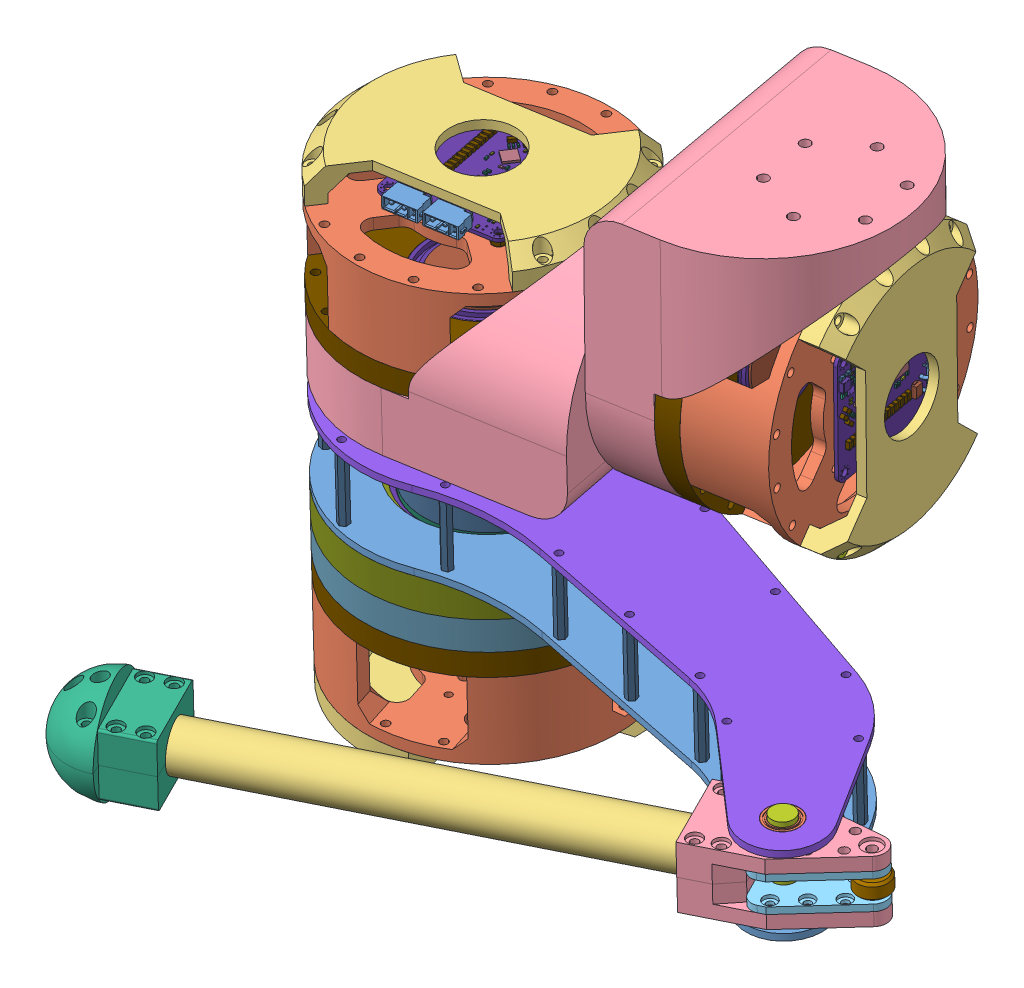
SolidWorks assembly leg, configuration Default. Lengths in mm.
Overall size (384.94 297.44 348.41).
919 component instances, 109 part files, 37 mates.
Components (placement in the parent):
- Leg_Upper - Copy-1: Leg_Upper - Copy [Default] at (49.985 212.2572 250.7825) x (0.920665 -0.018368 0.389921) z (-0.390312 -0.028778 0.920233) size (325 3 115)
- Bearing_10x15x4-1: Bearing_10x15x4 [Default] at (280.1626 209.664 348.3301) x (0.958733 -0.015014 0.283911) z (-0.284251 -0.030662 0.958259) size (15 4 15)
- Leg_lower-1: Leg_lower [Default] at (-5.0018 329.6044 276.4226) x (-0.005682 -0.999417 -0.033664) z (0.43435 -0.03279 0.900147) size (44.82 283.41 44.82)
  - Cacbon_20x18x200-1: Cacbon_20x18x200 [Default] at (99.8295 -0.5136 192.5214) size (20 215 20)
  - knee-1: knee [Default] at (99.8295 224.4864 192.5214) x (0 1 0) z (0 0 1) size (66 14 35)
  - knee - Copy-1: knee - Copy [Default] at (107.8295 224.4864 192.5214) x (0 1 0) z (0 0 1) size (44 3 35)
  - Foot-1: Foot [Default] at (99.8295 -0.5136 192.5214) x (0 1 0) z (0 0 1) size (42.41 22.41 44.82)
  - knee-3: knee [Default] at (99.8295 224.4864 192.5214) x (0 1 0) z (0 0 -1) size (66 14 35)
  - knee - Copy-3: knee - Copy [Default] at (91.8295 224.4864 192.5214) x (0 1 0) z (0 0 -1) size (44 3 35)
  - Foot-3: Foot [Default] at (99.8295 -0.5136 192.5214) x (0 1 0) z (0 0 -1) size (42.41 22.41 44.82)
  - m10-1: m10 [Default] at (99.8295 224.4864 192.5214) x (0 1 0) z (0 0 1) size (10 40 10)
- Leg_Upper-1: Leg_Upper [Default] at (50.1725 245.238 251.8934) x (0.920665 -0.018368 0.389921) z (-0.390312 -0.028778 0.920233) size (325 3 115)
- Bearing_10x15x4-2: Bearing_10x15x4 [Default] at (280.3444 241.6454 349.4074) x (0.969125 -0.013802 0.246184) z (0.246505 0.031226 -0.968638) size (15 4 15)
- Link_Rod-1: Link_Rod [Default] at (59.5022 231.363 216.6593) x (0.900993 -0.01972 0.433385) z (0.433797 0.027869 -0.90058) size (289 7 14)
- Link_rod_2-1: Link_rod_2 [Default] at (50.0418 222.2514 251.1191) x (0.965179 -0.014285 0.261198) z (-0.261527 -0.031008 0.964698) size (60 14.5 72)
- Cycloidal-1: Cycloidal [Default] at (89.0725 113.9575 154.6274) x (0.628302 -0.029758 0.7774) z (-0.777949 -0.016734 0.628105) size (162.63 86.6 162.63)
  - motor-X83008S.stp-1: motor-X83008S.stp [Default] at (44.8559 83.3915 132.8566) x (-0.221421 0 -0.975178) z (0 -1 0) size (114.7 114.7 37.62) (hidden)
    - base.stp-1: base.stp [Default] at (42.0794 12.0269 46.7342) size (91.6 91.6 15.61)
    - stator.stp-1: stator.stp [Default] at (42.0794 12.0269 33.1342) x (0.08493 -0.996387 0) z (0 0 1) size (83 83 8)
    - coil.stp-1: coil.stp [Default] at (39.5332 41.8984 37.1342) x (0.996387 0.08493 0) z (-0.08493 0.996387 0) size (4.4 10.2 10.5)
    - coil.stp-2: coil.stp [Default] at (34.3848 41.0025 37.1342) x (0.966502 0.256661 0) z (-0.256661 0.966502 0) size (4.4 10.2 10.5)
    - coil.stp-3: coil.stp [Default] at (29.4701 39.2261 37.1342) x (0.90725 0.420593 0) z (-0.420593 0.90725 0) size (4.4 10.2 10.5)
    - coil.stp-4: coil.stp [Default] at (24.9386 36.6233 37.1342) x (0.820431 0.571745 0) z (-0.571745 0.820431 0) size (4.4 10.2 10.5)
    - coil.stp-5: coil.stp [Default] at (20.9279 33.2732 37.1342) x (0.708685 0.705525 0) z (-0.705525 0.708685 0) size (4.4 10.2 10.5)
    - coil.stp-6: coil.stp [Default] at (17.5599 29.2775 37.1342) x (0.575405 0.817869 0) z (-0.817869 0.575405 0) size (4.4 10.2 10.5)
    - coil.stp-7: coil.stp [Default] at (14.9368 24.7576 37.1342) x (0.424642 0.905361 0) z (-0.905361 0.424642 0) size (4.4 10.2 10.5)
    - coil.stp-8: coil.stp [Default] at (13.1385 19.8509 37.1342) x (0.260976 0.965345 0) z (-0.965345 0.260976 0) size (4.4 10.2 10.5)
    - coil.stp-9: coil.stp [Default] at (12.2196 14.7066 37.1342) x (0.089381 0.995998 0) z (-0.995998 0.089381 0) size (4.4 10.2 10.5)
    - coil.stp-10: coil.stp [Default] at (12.2079 9.4807 37.1342) x (-0.08493 0.996387 0) z (-0.996387 -0.08493 0) size (4.4 10.2 10.5)
    - coil.stp-11: coil.stp [Default] at (13.1039 4.3323 37.1342) x (-0.256661 0.966502 0) z (-0.966502 -0.256661 0) size (4.4 10.2 10.5)
    - coil.stp-12: coil.stp [Default] at (14.8802 -0.5824 37.1342) x (-0.420593 0.90725 0) z (-0.90725 -0.420593 0) size (4.4 10.2 10.5)
    - coil.stp-13: coil.stp [Default] at (17.483 -5.1139 37.1342) x (-0.571745 0.820431 0) z (-0.820431 -0.571745 0) size (4.4 10.2 10.5)
    - coil.stp-14: coil.stp [Default] at (20.8332 -9.1246 37.1342) x (-0.705525 0.708685 0) z (-0.708685 -0.705525 0) size (4.4 10.2 10.5)
    - coil.stp-15: coil.stp [Default] at (24.8289 -12.4926 37.1342) x (-0.817869 0.575405 0) z (-0.575405 -0.817869 0) size (4.4 10.2 10.5)
    - coil.stp-16: coil.stp [Default] at (29.3487 -15.1157 37.1342) x (-0.905361 0.424642 0) z (-0.424642 -0.905361 0) size (4.4 10.2 10.5)
    - coil.stp-17: coil.stp [Default] at (34.2554 -16.914 37.1342) x (-0.965345 0.260976 0) z (-0.260976 -0.965345 0) size (4.4 10.2 10.5)
    - coil.stp-18: coil.stp [Default] at (39.3998 -17.8329 37.1342) x (-0.995998 0.089381 0) z (-0.089381 -0.995998 0) size (4.4 10.2 10.5)
    - coil.stp-19: coil.stp [Default] at (44.6256 -17.8446 37.1342) x (-0.996387 -0.08493 0) z (0.08493 -0.996387 0) size (4.4 10.2 10.5)
    - coil.stp-20: coil.stp [Default] at (49.7741 -16.9486 37.1342) x (-0.966502 -0.256661 0) z (0.256661 -0.966502 0) size (4.4 10.2 10.5)
    - coil.stp-21: coil.stp [Default] at (54.6887 -15.1723 37.1342) x (-0.90725 -0.420593 0) z (0.420593 -0.90725 0) size (4.4 10.2 10.5)
    - coil.stp-22: coil.stp [Default] at (59.2202 -12.5695 37.1342) x (-0.820431 -0.571745 0) z (0.571745 -0.820431 0) size (4.4 10.2 10.5)
    - coil.stp-23: coil.stp [Default] at (63.2309 -9.2193 37.1342) x (-0.708685 -0.705525 0) z (0.705525 -0.708685 0) size (4.4 10.2 10.5)
    - coil.stp-24: coil.stp [Default] at (66.599 -5.2236 37.1342) x (-0.575405 -0.817869 0) z (0.817869 -0.575405 0) size (4.4 10.2 10.5)
    - coil.stp-25: coil.stp [Default] at (69.222 -0.7038 37.1342) x (-0.424642 -0.905361 0) z (0.905361 -0.424642 0) size (4.4 10.2 10.5)
    - coil.stp-26: coil.stp [Default] at (71.0203 4.2029 37.1342) x (-0.260976 -0.965345 0) z (0.965345 -0.260976 0) size (4.4 10.2 10.5)
    - coil.stp-27: coil.stp [Default] at (71.9392 9.3473 37.1342) x (-0.089381 -0.995998 0) z (0.995998 -0.089381 0) size (4.4 10.2 10.5)
    - coil.stp-28: coil.stp [Default] at (71.9509 14.5731 37.1342) x (0.08493 -0.996387 0) z (0.996387 0.08493 0) size (4.4 10.2 10.5)
    - coil.stp-29: coil.stp [Default] at (71.055 19.7216 37.1342) x (0.256661 -0.966502 0) z (0.966502 0.256661 0) size (4.4 10.2 10.5)
    - coil.stp-30: coil.stp [Default] at (69.2786 24.6362 37.1342) x (0.420593 -0.90725 0) z (0.90725 0.420593 0) size (4.4 10.2 10.5)
    - coil.stp-31: coil.stp [Default] at (66.6758 29.1677 37.1342) x (0.571745 -0.820431 0) z (0.820431 0.571745 0) size (4.4 10.2 10.5)
    - coil.stp-32: coil.stp [Default] at (63.3257 33.1785 37.1342) x (0.705525 -0.708685 0) z (0.708685 0.705525 0) size (4.4 10.2 10.5)
    - coil.stp-33: coil.stp [Default] at (59.33 36.5465 37.1342) x (0.817869 -0.575405 0) z (0.575405 0.817869 0) size (4.4 10.2 10.5)
    - coil.stp-34: coil.stp [Default] at (54.8101 39.1695 37.1342) x (0.905361 -0.424642 0) z (0.424642 0.905361 0) size (4.4 10.2 10.5)
    - coil.stp-35: coil.stp [Default] at (49.9034 40.9678 37.1342) x (0.965345 -0.260976 0) z (0.260976 0.965345 0) size (4.4 10.2 10.5)
    - coil.stp-36: coil.stp [Default] at (44.759 41.8868 37.1342) x (0.995998 -0.089381 0) z (0.089381 0.995998 0) size (4.4 10.2 10.5)
    - rotor.stp-1: rotor.stp [Default] at (42.0794 12.0269 42.1342) x (-0.293442 0.955977 0) z (0 0 -1) size (91.8 91.8 12)
    - outrunner.stp-1: outrunner.stp [Default] at (42.0794 12.0269 30.1342) x (-0.254711 0.967017 0) z (-0.967017 -0.254711 0) size (91.8 17.01 91.8)
    - screw-mount.stp-1: screw-mount.stp [Default] at (38.1314 27.0157 27.1342) x (1 0 0) z (0 0 -1) size (7 7 6.5)
    - screw-mount.stp-2: screw-mount.stp [Default] at (27.0906 8.0789 27.1342) x (1 0 0) z (0 0 -1) size (7 7 6.5)
    - screw-mount.stp-3: screw-mount.stp [Default] at (57.0682 15.9749 27.1342) x (1 0 0) z (0 0 -1) size (7 7 6.5)
    - screw-mount.stp-4: screw-mount.stp [Default] at (46.0274 -2.9618 27.1342) x (1 0 0) z (0 0 -1) size (7 7 6.5)
    - 6702ZZ-bearing-15x21x4.stp-1: 6702ZZ-bearing-15x21x4.stp [Default] at (42.0794 12.0269 43.7342) x (1 0 0) z (0 -1 0) size (21 4 21)
    - 6702ZZ-bearing-15x21x4.stp-2: 6702ZZ-bearing-15x21x4.stp [Default] at (42.0794 12.0269 35.1342) x (1 0 0) z (0 1 0) size (21 4 21)
    - shaft.stp-1: shaft.stp [Default] at (42.0794 12.0269 20.1342) size (16 16 31.6)
    - fix-screw.stp-1: fix-screw.stp [Default] at (42.0794 12.0269 51.7342) x (1 0 0) z (0 0 -1) size (19.67 18.96 12.02)
  - Base_Plate-1: Base_Plate [Default] at (47.267 63.2573 89.1587) x (-0.03427 0 0.999413) z (-0.999413 0 -0.03427) size (39.8 11 39.8)
  - Eccentric_Shaft-1: Eccentric_Shaft [Default] at (54.4098 67.9165 103.5023) x (-0.999413 0 -0.03427) z (0.03427 0 -0.999413) size (20 17 17)
    - Eccentric_Shaft_bot-1: Eccentric_Shaft_bot [Default] at (7.6302 12.3409 14.0904) x (1 0 0) z (0 0 -1) size (17 6 17)
    - Eccentric_Shaft_bot-2: Eccentric_Shaft_bot [Default] at (7.6302 12.3409 14.0904) x (-1 0 0) z (0 0 -1) size (17 6 17)
    - Eccentric_Shaft_top-1: Eccentric_Shaft_top [Default] at (7.6302 18.3409 14.0904) x (-1 0 0) z (0 0 -1) size (17 5 17)
  - Ring_Pin_Housing-1: Ring_Pin_Housing [Default] at (47.267 74.2573 89.1587) x (0.707107 0 -0.707107) z (0.707107 0 0.707107) size (115 13 115)
  - Output_Shaft-1: Output_Shaft [Default] at (47.267 87.2573 89.1587) x (0.353379 0 -0.93548) z (0.93548 0 0.353379) size (70 14 70)
  - Cover-1: Cover [Default] at (47.267 87.2573 89.1587) x (0.707107 0 -0.707107) z (0.707107 0 0.707107) size (115 14.4 115)
  - radial ball bearing_68_iso-39: radial ball bearing_68_iso [ISO 15 RBB - 1860 - 32,SI,NC,32_68] at (47.267 94.2573 89.1587) x (0 1 0) z (-0.131235 0 0.991351) size (10 78 78)
  - radial ball bearing_68_iso-40: radial ball bearing_68_iso [ISO 15 RBB - 1840 - 32,SI,NC,32_68] at (47.267 70.7573 89.1587) x (0 1 0) z (0.001003 0 0.999999) size (7 52 52)
  - Base_plate_2-1: Base_plate_2 [Default] at (47.267 64.2573 89.1587) x (0.707107 0 -0.707107) z (0.707107 0 0.707107) size (115 10 115)
  - m13_bearing-31: m13_bearing [Default] at (-10.7414 95.4081 67.0593) x (0.227678 0 0.973736) z (0.973736 0 -0.227678) size (13 16 13)
    - m6-1: m6 [Default] at (8.4921 2.5508 14.8914) size (6 16 6)
    - radial ball bearing_68_iso-1: radial ball bearing_68_iso [ISO 15 RBB - 286 - 10,SI,NC,10_68] at (8.4921 16.0508 14.8914) x (0 1 0) z (0 0 1) size (5 13 13)
    - radial ball bearing_68_iso-2: radial ball bearing_68_iso [ISO 15 RBB - 286 - 10,SI,NC,10_68] at (8.4921 11.0508 14.8914) x (0 1 0) z (0 0 1) size (5 13 13)
  - m13_bearing-32: m13_bearing [Default] at (-14.1668 95.4081 84.2801) x (0.227678 0 0.973736) z (0.973736 0 -0.227678) size (13 16 13)
    - m6-1: m6 [Default] at (8.4921 2.5508 14.8914) size (6 16 6)
    - radial ball bearing_68_iso-1: radial ball bearing_68_iso [ISO 15 RBB - 286 - 10,SI,NC,10_68] at (8.4921 16.0508 14.8914) x (0 1 0) z (0 0 1) size (5 13 13)
    - radial ball bearing_68_iso-2: radial ball bearing_68_iso [ISO 15 RBB - 286 - 10,SI,NC,10_68] at (8.4921 11.0508 14.8914) x (0 1 0) z (0 0 1) size (5 13 13)
  - m13_bearing-34: m13_bearing [Default] at (13.6125 95.5581 125.8547) x (0.227678 0 0.973736) z (0.973736 0 -0.227678) size (13 16 13)
    - m6-1: m6 [Default] at (8.4921 2.5508 14.8914) size (6 16 6)
    - radial ball bearing_68_iso-1: radial ball bearing_68_iso [ISO 15 RBB - 286 - 10,SI,NC,10_68] at (8.4921 16.0508 14.8914) x (0 1 0) z (0 0 1) size (5 13 13)
    - radial ball bearing_68_iso-2: radial ball bearing_68_iso [ISO 15 RBB - 286 - 10,SI,NC,10_68] at (8.4921 11.0508 14.8914) x (0 1 0) z (0 0 1) size (5 13 13)
  - m13_bearing-35: m13_bearing [Default] at (-0.9866 95.4081 116.0999) x (0.227678 0 0.973736) z (0.973736 0 -0.227678) size (13 16 13)
    - m6-1: m6 [Default] at (8.4921 2.5508 14.8914) size (6 16 6)
    - radial ball bearing_68_iso-1: radial ball bearing_68_iso [ISO 15 RBB - 286 - 10,SI,NC,10_68] at (8.4921 16.0508 14.8914) x (0 1 0) z (0 0 1) size (5 13 13)
    - radial ball bearing_68_iso-2: radial ball bearing_68_iso [ISO 15 RBB - 286 - 10,SI,NC,10_68] at (8.4921 11.0508 14.8914) x (0 1 0) z (0 0 1) size (5 13 13)
  - m13_bearing-36: m13_bearing [Default] at (-10.7414 95.5581 101.5009) x (0.227678 0 0.973736) z (0.973736 0 -0.227678) size (13 16 13)
    - m6-1: m6 [Default] at (8.4921 2.5508 14.8914) size (6 16 6)
    - radial ball bearing_68_iso-1: radial ball bearing_68_iso [ISO 15 RBB - 286 - 10,SI,NC,10_68] at (8.4921 16.0508 14.8914) x (0 1 0) z (0 0 1) size (5 13 13)
    - radial ball bearing_68_iso-2: radial ball bearing_68_iso [ISO 15 RBB - 286 - 10,SI,NC,10_68] at (8.4921 11.0508 14.8914) x (0 1 0) z (0 0 1) size (5 13 13)
  - m13_bearing-1: m13_bearing [Default] at (-0.8801 95.4081 62.5627) x (0.736525 0 0.676411) z (0.676411 0 -0.736525) size (13 16 13)
    - m6-1: m6 [Default] at (8.4921 2.5508 14.8914) size (6 16 6)
    - radial ball bearing_68_iso-1: radial ball bearing_68_iso [ISO 15 RBB - 286 - 10,SI,NC,10_68] at (8.4921 16.0508 14.8914) x (0 1 0) z (0 0 1) size (5 13 13)
    - radial ball bearing_68_iso-2: radial ball bearing_68_iso [ISO 15 RBB - 286 - 10,SI,NC,10_68] at (8.4921 11.0508 14.8914) x (0 1 0) z (0 0 1) size (5 13 13)
  - m13_bearing-2: m13_bearing [Default] at (48.6831 95.4081 124.0939) x (0.120271 0 0.992741) z (0.992741 0 -0.120271) size (13 16 13)
    - m6-1: m6 [Default] at (8.4921 2.5508 14.8914) size (6 16 6)
    - radial ball bearing_68_iso-1: radial ball bearing_68_iso [ISO 15 RBB - 286 - 10,SI,NC,10_68] at (8.4921 16.0508 14.8914) x (0 1 0) z (0 0 1) size (5 13 13)
    - radial ball bearing_68_iso-2: radial ball bearing_68_iso [ISO 15 RBB - 286 - 10,SI,NC,10_68] at (8.4921 11.0508 14.8914) x (0 1 0) z (0 0 1) size (5 13 13)
  - m13_bearing-3: m13_bearing [Default] at (32.7832 95.4081 34.9886) x (-0.046141 0 0.998935) z (0.998935 0 0.046141) size (13 16 13)
    - m6-1: m6 [Default] at (8.4921 2.5508 14.8914) size (6 16 6)
    - radial ball bearing_68_iso-1: radial ball bearing_68_iso [ISO 15 RBB - 286 - 10,SI,NC,10_68] at (8.4921 16.0508 14.8914) x (0 1 0) z (0 0 1) size (5 13 13)
    - radial ball bearing_68_iso-2: radial ball bearing_68_iso [ISO 15 RBB - 286 - 10,SI,NC,10_68] at (8.4921 11.0508 14.8914) x (0 1 0) z (0 0 1) size (5 13 13)
  - m13_bearing-4: m13_bearing [Default] at (77.1902 95.4081 81.0003) x (0.022268 0 0.999752) z (0.999752 0 -0.022268) size (13 16 13)
    - m6-1: m6 [Default] at (8.4921 2.5508 14.8914) size (6 16 6)
    - radial ball bearing_68_iso-1: radial ball bearing_68_iso [ISO 15 RBB - 286 - 10,SI,NC,10_68] at (8.4921 16.0508 14.8914) x (0 1 0) z (0 0 1) size (5 13 13)
    - radial ball bearing_68_iso-2: radial ball bearing_68_iso [ISO 15 RBB - 286 - 10,SI,NC,10_68] at (8.4921 11.0508 14.8914) x (0 1 0) z (0 0 1) size (5 13 13)
  - m13_bearing-5: m13_bearing [Default] at (73.474 95.4081 98.7828) x (0.059133 0 0.99825) z (0.99825 0 -0.059133) size (13 16 13)
    - m6-1: m6 [Default] at (8.4921 2.5508 14.8914) size (6 16 6)
    - radial ball bearing_68_iso-1: radial ball bearing_68_iso [ISO 15 RBB - 286 - 10,SI,NC,10_68] at (8.4921 16.0508 14.8914) x (0 1 0) z (0 0 1) size (5 13 13)
    - radial ball bearing_68_iso-2: radial ball bearing_68_iso [ISO 15 RBB - 286 - 10,SI,NC,10_68] at (8.4921 11.0508 14.8914) x (0 1 0) z (0 0 1) size (5 13 13)
  - m13_bearing-6: m13_bearing [Default] at (12.9248 95.4081 46.7315) x (0.451561 0 0.89224) z (0.89224 0 -0.451561) size (13 16 13)
    - m6-1: m6 [Default] at (8.4921 2.5508 14.8914) size (6 16 6)
    - radial ball bearing_68_iso-1: radial ball bearing_68_iso [ISO 15 RBB - 286 - 10,SI,NC,10_68] at (8.4921 16.0508 14.8914) x (0 1 0) z (0 0 1) size (5 13 13)
    - radial ball bearing_68_iso-2: radial ball bearing_68_iso [ISO 15 RBB - 286 - 10,SI,NC,10_68] at (8.4921 11.0508 14.8914) x (0 1 0) z (0 0 1) size (5 13 13)
  - m13_bearing-7: m13_bearing [Default] at (56.6452 95.4081 32.3406) x (-0.545813 0 0.837907) z (0.837907 0 0.545813) size (13 16 13)
    - m6-1: m6 [Default] at (8.4921 2.5508 14.8914) size (6 16 6)
    - radial ball bearing_68_iso-1: radial ball bearing_68_iso [ISO 15 RBB - 286 - 10,SI,NC,10_68] at (8.4921 16.0508 14.8914) x (0 1 0) z (0 0 1) size (5 13 13)
    - radial ball bearing_68_iso-2: radial ball bearing_68_iso [ISO 15 RBB - 286 - 10,SI,NC,10_68] at (8.4921 11.0508 14.8914) x (0 1 0) z (0 0 1) size (5 13 13)
  - m13_bearing-8: m13_bearing [Default] at (63.0373 95.4081 51.3153) x (0.158553 0 0.98735) z (0.98735 0 -0.158553) size (13 16 13)
    - m6-1: m6 [Default] at (8.4921 2.5508 14.8914) size (6 16 6)
    - radial ball bearing_68_iso-1: radial ball bearing_68_iso [ISO 15 RBB - 286 - 10,SI,NC,10_68] at (8.4921 16.0508 14.8914) x (0 1 0) z (0 0 1) size (5 13 13)
    - radial ball bearing_68_iso-2: radial ball bearing_68_iso [ISO 15 RBB - 286 - 10,SI,NC,10_68] at (8.4921 11.0508 14.8914) x (0 1 0) z (0 0 1) size (5 13 13)
  - m13_bearing-9: m13_bearing [Default] at (83.8577 95.4081 55.5358) x (-0.687134 0 0.72653) z (0.72653 0 0.687134) size (13 16 13)
    - m6-1: m6 [Default] at (8.4921 2.5508 14.8914) size (6 16 6)
    - radial ball bearing_68_iso-1: radial ball bearing_68_iso [ISO 15 RBB - 286 - 10,SI,NC,10_68] at (8.4921 16.0508 14.8914) x (0 1 0) z (0 0 1) size (5 13 13)
    - radial ball bearing_68_iso-2: radial ball bearing_68_iso [ISO 15 RBB - 286 - 10,SI,NC,10_68] at (8.4921 11.0508 14.8914) x (0 1 0) z (0 0 1) size (5 13 13)
  - m13_bearing-11: m13_bearing [Default] at (30.1977 95.4081 135.7424) x (0.57351 0 0.819198) z (0.819198 0 -0.57351) size (13 16 13)
    - m6-1: m6 [Default] at (8.4921 2.5508 14.8914) size (6 16 6)
    - radial ball bearing_68_iso-1: radial ball bearing_68_iso [ISO 15 RBB - 286 - 10,SI,NC,10_68] at (8.4921 16.0508 14.8914) x (0 1 0) z (0 0 1) size (5 13 13)
    - radial ball bearing_68_iso-2: radial ball bearing_68_iso [ISO 15 RBB - 286 - 10,SI,NC,10_68] at (8.4921 11.0508 14.8914) x (0 1 0) z (0 0 1) size (5 13 13)
  - m13_bearing-12: m13_bearing [Default] at (62.8861 95.4081 115.3744) x (0.184178 0 0.982893) z (0.982893 0 -0.184178) size (13 16 13)
    - m6-1: m6 [Default] at (8.4921 2.5508 14.8914) size (6 16 6)
    - radial ball bearing_68_iso-1: radial ball bearing_68_iso [ISO 15 RBB - 286 - 10,SI,NC,10_68] at (8.4921 16.0508 14.8914) x (0 1 0) z (0 0 1) size (5 13 13)
    - radial ball bearing_68_iso-2: radial ball bearing_68_iso [ISO 15 RBB - 286 - 10,SI,NC,10_68] at (8.4921 11.0508 14.8914) x (0 1 0) z (0 0 1) size (5 13 13)
  - M3x4x4.2_brass_insert-22: M3x4x4.2_brass_insert [Default] at (47.1299 63.2573 93.1563) x (0.984609 0 -0.174769) z (0.174769 0 0.984609) size (4 4 4)
  - M3x4x4.2_brass_insert-23: M3x4x4.2_brass_insert [Default] at (47.4041 63.2573 85.161) x (0.984609 0 -0.174769) z (0.174769 0 0.984609) size (4 4 4)
  - radial ball bearing_68_iso-44: radial ball bearing_68_iso [ISO 15 RBB - 1715 - 26,SI,NC,26_68] at (45.7679 83.7573 89.1073) x (0 1 0) z (-0.714953 0 -0.699173) size (4 21 21)
  - radial ball bearing_68_iso-45: radial ball bearing_68_iso [ISO 15 RBB - 1715 - 26,SI,NC,26_68] at (47.267 89.2573 89.1587) x (0 1 0) z (0.999483 0 -0.032163) size (4 21 21)
  - radial ball bearing_68_iso-46: radial ball bearing_68_iso [ISO 15 RBB - 1715 - 26,SI,NC,26_68] at (48.7661 76.2573 89.2101) x (0 -1 0) z (0.546944 0 -0.837169) size (4 21 21)
  - socket button head screw_iso-37: socket button head screw_iso [ISO 7380 - M4 x 12 - 12N] at (79.0868 62.0573 57.3389) x (0 1 0) z (-0.709975 0 0.704227) size (14.2 7.6 7.6)
  - socket button head screw_iso-38: socket button head screw_iso [ISO 7380 - M4 x 12 - 12N] at (64.4877 62.0573 130.7332) x (0 1 0) z (-0.724148 0 0.689645) size (14.2 7.6 7.6)
  - foc-motor-controller.step-1: foc-motor-controller.step [Default] at (47.267 27.2573 89.1587) x (0.382683 0 0.92388) z (0 -1 0) size (57.23 50 8.13)
    - RTA0040B.step-1: RTA0040B.step [Default] at (12.5014 -1.6986 1.595) x (-0.707107 -0.707107 0) z (0 0 1) size (6 6 1)
      - FRAME.step-1: FRAME.step [Default] x (1 0 0) z (0 -1 0) size (6 0.2 6)
        - SOLID.step-1: SOLID.step [Default] at origin size (0.4 0.2 0.22)
        - SOLID-0.step-1: SOLID-0.step [Default] at origin size (0.4 0.2 0.22)
        - SOLID-1.step-1: SOLID-1.step [Default] at origin size (0.4 0.2 0.22)
        - SOLID-2.step-1: SOLID-2.step [Default] at origin size (0.4 0.2 0.22)
        - SOLID-3.step-1: SOLID-3.step [Default] at origin size (0.4 0.2 0.22)
        - SOLID-4.step-1: SOLID-4.step [Default] at origin size (0.4 0.2 0.22)
        - SOLID-5.step-1: SOLID-5.step [Default] at origin size (0.4 0.2 0.22)
        - SOLID-6.step-1: SOLID-6.step [Default] at origin size (0.4 0.2 0.22)
        - SOLID-7.step-1: SOLID-7.step [Default] at origin size (0.4 0.2 0.22)
        - SOLID-8.step-1: SOLID-8.step [Default] at origin size (0.4 0.2 0.22)
        - SOLID-9.step-1: SOLID-9.step [Default] at origin size (0.22 0.2 0.4)
        - SOLID-10.step-1: SOLID-10.step [Default] at origin size (0.22 0.2 0.4)
        - SOLID-11.step-1: SOLID-11.step [Default] at origin size (0.22 0.2 0.4)
        - SOLID-12.step-1: SOLID-12.step [Default] at origin size (0.22 0.2 0.4)
        - SOLID-13.step-1: SOLID-13.step [Default] at origin size (0.22 0.2 0.4)
        - SOLID-14.step-1: SOLID-14.step [Default] at origin size (0.22 0.2 0.4)
        - SOLID-15.step-1: SOLID-15.step [Default] at origin size (0.22 0.2 0.4)
        - SOLID-16.step-1: SOLID-16.step [Default] at origin size (0.22 0.2 0.4)
        - SOLID-17.step-1: SOLID-17.step [Default] at origin size (4.15 0.2 4.15)
        - SOLID-18.step-1: SOLID-18.step [Default] at origin size (0.28 0.1 0.28)
        - SOLID-19.step-1: SOLID-19.step [Default] at origin size (0.28 0.1 0.28)
        - SOLID-20.step-1: SOLID-20.step [Default] at origin size (0.28 0.1 0.28)
        - SOLID-21.step-1: SOLID-21.step [Default] at origin size (0.28 0.1 0.28)
        - SOLID-22.step-1: SOLID-22.step [Default] at origin size (0.4 0.2 0.22)
        - SOLID-23.step-1: SOLID-23.step [Default] at origin size (0.4 0.2 0.22)
        - SOLID-24.step-1: SOLID-24.step [Default] at origin size (0.4 0.2 0.22)
        - SOLID-25.step-1: SOLID-25.step [Default] at origin size (0.4 0.2 0.22)
        - SOLID-26.step-1: SOLID-26.step [Default] at origin size (0.4 0.2 0.22)
        - SOLID-27.step-1: SOLID-27.step [Default] at origin size (0.4 0.2 0.22)
        - SOLID-28.step-1: SOLID-28.step [Default] at origin size (0.4 0.2 0.22)
        - SOLID-29.step-1: SOLID-29.step [Default] at origin size (0.4 0.2 0.22)
        - SOLID-30.step-1: SOLID-30.step [Default] at origin size (0.4 0.2 0.22)
        - SOLID-31.step-1: SOLID-31.step [Default] at origin size (0.4 0.2 0.22)
        - SOLID-32.step-1: SOLID-32.step [Default] at origin size (0.22 0.2 0.4)
        - SOLID-33.step-1: SOLID-33.step [Default] at origin size (0.22 0.2 0.4)
        - SOLID-34.step-1: SOLID-34.step [Default] at origin size (0.22 0.2 0.4)
        - SOLID-35.step-1: SOLID-35.step [Default] at origin size (0.22 0.2 0.4)
        - SOLID-36.step-1: SOLID-36.step [Default] at origin size (0.22 0.2 0.4)
        - SOLID-37.step-1: SOLID-37.step [Default] at origin size (0.22 0.2 0.4)
        - SOLID-38.step-1: SOLID-38.step [Default] at origin size (0.22 0.2 0.4)
        - SOLID-39.step-1: SOLID-39.step [Default] at origin size (0.22 0.2 0.4)
        - SOLID-40.step-1: SOLID-40.step [Default] at origin size (0.22 0.2 0.4)
        - SOLID-41.step-1: SOLID-41.step [Default] at origin size (0.22 0.2 0.4)
        - SOLID-42.step-1: SOLID-42.step [Default] at origin size (0.22 0.2 0.4)
        - SOLID-43.step-1: SOLID-43.step [Default] at origin size (0.22 0.2 0.4)
      - BODY.step-1: BODY.step [Default] at (0 0 0.025) x (1 0 0) z (0 -1 0) size (6 0.97 6)
    - Resonator_SMD_Murata_CSTxExxV-3Pin_3.0x1.1mm.step-1: Resonator_SMD_Murata_CSTxExxV-3Pin_3.0x1.1mm.step [Default] at (1.8 -7 1.595) x (0 1 0) z (0 0 1) size (3.2 1.35 0.9)
    - C_0603_1608Metric.step-1: C_0603_1608Metric.step [Default] at (6.2 -16.8 1.595) x (0 -1 0) z (0 0 1) size (1.6 0.8 0.8)
    - R_0603_1608Metric.step-1: R_0603_1608Metric.step [Default] at (11.8 -7.375 1.595) x (0 1 0) z (0 0 1) size (1.6 0.8 0.45)
    - R_0603_1608Metric.step-2: R_0603_1608Metric.step [Default] at (13.8 -16.8 1.595) x (0 1 0) z (0 0 1) size (1.6 0.8 0.45)
    - R_0603_1608Metric.step-3: R_0603_1608Metric.step [Default] at (18.1 -5.36 1.595) size (1.6 0.8 0.45)
    - C_0603_1608Metric.step-2: C_0603_1608Metric.step [Default] at (2.6 -0.5 1.595) x (0 -1 0) z (0 0 1) size (1.6 0.8 0.8)
    - R_0603_1608Metric.step-4: R_0603_1608Metric.step [Default] at (14.6 -11.3 1.595) x (0 1 0) z (0 0 1) size (1.6 0.8 0.45)
    - L_APV_ANR4020.step-1: L_APV_ANR4020.step [Default] at (22.3 -13.7 1.595) x (0 -1 0) z (0 0 1) size (4.02 4 2)
    - C_0603_1608Metric.step-3: C_0603_1608Metric.step [Default] at (0.3 -12.6 1.595) x (-1 0 0) z (0 0 1) size (1.6 0.8 0.8)
    - C_1206_3216Metric.step-1: C_1206_3216Metric.step [Default] at (15.7 11 1.595) x (0 1 0) z (0 0 1) size (3.2 1.6 1.6)
    - C_0603_1608Metric.step-4: C_0603_1608Metric.step [Default] at (0.3 -9.6 1.595) size (1.6 0.8 0.8)
    - R_0603_1608Metric.step-5: R_0603_1608Metric.step [Default] at (12.3 -16.8 1.595) x (0 1 0) z (0 0 1) size (1.6 0.8 0.45)
    - C_0603_1608Metric.step-5: C_0603_1608Metric.step [Default] at (-0.3 -16.6 1.595) x (0 1 0) z (0 0 1) size (1.6 0.8 0.8)
    - R_0603_1608Metric.step-6: R_0603_1608Metric.step [Default] at (10.9 4.1 1.595) size (1.6 0.8 0.45)
    - C_1206_3216Metric.step-2: C_1206_3216Metric.step [Default] at (6.3 11 1.595) x (0 1 0) z (0 0 1) size (3.2 1.6 1.6)
    - XT30PW_2_2_-M.G.B.step-1: XT30PW_2_2_-M.G.B.step [Default] at (-20.5 9.5 1.595) x (0 -1 0) z (-1 0 0) size (15.5 7.1 12.53)
    - R_0603_1608Metric.step-7: R_0603_1608Metric.step [Default] at (0.3 -11.1 1.595) size (1.6 0.8 0.45)
    - C_0603_1608Metric.step-6: C_0603_1608Metric.step [Default] at (19 -0.4 1.595) x (-0.707107 -0.707107 0) z (0 0 1) size (1.6 0.8 0.8)
    - C_1206_3216Metric.step-3: C_1206_3216Metric.step [Default] at (13.3 11 1.595) x (0 1 0) z (0 0 1) size (3.2 1.6 1.6)
    - R_0603_1608Metric.step-8: R_0603_1608Metric.step [Default] at (10.2 -7.375 1.595) x (0 -1 0) z (0 0 1) size (1.6 0.8 0.45)
    - JST_GH_SM08B-GHS-TB_1x08-1MP_P1.25mm_Horizontal.step-1: JST_GH_SM08B-GHS-TB_1x08-1MP_P1.25mm_Horizontal.step [Default] at (10 -22 1.595) size (13.25 4.95 4.25)
    - C_1206_3216Metric.step-4: C_1206_3216Metric.step [Default] at (-12.3 11 1.595) x (0 1 0) z (0 0 1) size (3.2 1.6 1.6)
    - JST_GH_SM06B-GHS-TB_1x06-1MP_P1.25mm_Horizontal.step-1: JST_GH_SM06B-GHS-TB_1x06-1MP_P1.25mm_Horizontal.step [Default] at (-4.3 -22 1.595) size (10.75 4.95 4.25)
    - C_0603_1608Metric.step-7: C_0603_1608Metric.step [Default] at (7.3 -4.5 1.595) x (-1 0 0) z (0 0 1) size (1.6 0.8 0.8)
    - R_0603_1608Metric.step-9: R_0603_1608Metric.step [Default] at (18.1 -3.86 1.595) x (-1 0 0) z (0 0 1) size (1.6 0.8 0.45)
    - C_1206_3216Metric.step-5: C_1206_3216Metric.step [Default] at (22.6794 -1.2206 1.595) x (0.707107 -0.707107 0) z (0 0 1) size (3.2 1.6 1.6)
    - R_Array_Convex_4x0402.step-1: R_Array_Convex_4x0402.step [Default] at (6.8 -2.5 1.595) size (1 2 0.35)
    - R_0603_1608Metric.step-10: R_0603_1608Metric.step [Default] at (7.7 -16.8 1.595) x (0 -1 0) z (0 0 1) size (1.6 0.8 0.45)
    - C_1206_3216Metric.step-6: C_1206_3216Metric.step [Default] at (8.7 11 1.595) x (0 1 0) z (0 0 1) size (3.2 1.6 1.6)
    - C_0603_1608Metric.step-8: C_0603_1608Metric.step [Default] at (16.1 -11.3 1.595) x (0 1 0) z (0 0 1) size (1.6 0.8 0.8)
    - SOT-23-5.step-1: SOT-23-5.step [Default] at (-3.1 -16.6 1.595) x (-1 0 0) z (0 0 1) size (2.8 2.9 1.55)
    - C_0603_1608Metric.step-9: C_0603_1608Metric.step [Default] at (17.8 -13.6 1.595) size (1.6 0.8 0.8)
    - R_0603_1608Metric.step-11: R_0603_1608Metric.step [Default] at (-11.5 -20.3875 1.595) x (0 -1 0) z (0 0 1) size (1.6 0.8 0.45)
    - C_0603_1608Metric.step-10: C_0603_1608Metric.step [Default] at (-12.4 2.3 1.595) x (0 1 0) z (0 0 1) size (1.6 0.8 0.8)
    - C_1206_3216Metric.step-7: C_1206_3216Metric.step [Default] at (18 11 1.595) x (0 1 0) z (0 0 1) size (3.2 1.6 1.6)
    - R_0603_1608Metric.step-12: R_0603_1608Metric.step [Default] at (-10.8105 -14.9971 1.595) x (-1 0 0) z (0 0 1) size (1.6 0.8 0.45)
    - C_0603_1608Metric.step-11: C_0603_1608Metric.step [Default] at (-13.8 -9.4 1.595) x (-1 0 0) z (0 0 1) size (1.6 0.8 0.8)
    - R_0603_1608Metric.step-13: R_0603_1608Metric.step [Default] at (-23.15 -14.5 1.595) x (-1 0 0) z (0 0 1) size (1.6 0.8 0.45)
    - C_0603_1608Metric.step-12: C_0603_1608Metric.step [Default] at (1.1 -0.2 1.595) x (0 1 0) z (0 0 1) size (1.6 0.8 0.8)
    - D_0805_2012Metric.step-1: D_0805_2012Metric.step [Default] at (22.9 -9.6 1.595) x (0 1 0) z (0 0 1) size (2 1.27 0.8)
    - C_0603_1608Metric.step-13: C_0603_1608Metric.step [Default] at (-7.8 3.775 1.595) x (0 -1 0) z (0 0 1) size (1.6 0.8 0.8)
    - R_0603_1608Metric.step-14: R_0603_1608Metric.step [Default] at (-6.4 -12.825 1.595) x (0 1 0) z (0 0 1) size (1.6 0.8 0.45)
    - L_0603_1608Metric.step-1: L_0603_1608Metric.step [Default] at (-10.1 3 1.595) size (1.6 0.8 0.8)
    - C_0603_1608Metric.step-14: C_0603_1608Metric.step [Default] at (17.9 0.7 1.595) x (-0.707107 -0.707107 0) z (0 0 1) size (1.6 0.8 0.8)
    - HVSSOP-10.step-1: HVSSOP-10.step [Default] at (18.6 -9.6 1.595) x (0 -1 0) z (-1 0 0) size (4.9 1.1 3)
    - C_0603_1608Metric.step-15: C_0603_1608Metric.step [Default] at (7.9 4.1 1.595) x (-1 0 0) z (0 0 1) size (1.6 0.8 0.8)
    - C_0603_1608Metric.step-16: C_0603_1608Metric.step [Default] at (21.1 -9.6 1.595) x (0 -1 0) z (0 0 1) size (1.6 0.8 0.8)
    - R_0603_1608Metric.step-15: R_0603_1608Metric.step [Default] at (-10.8105 -11.9971 1.595) x (-1 0 0) z (0 0 1) size (1.6 0.8 0.45)
    - R_0603_1608Metric.step-16: R_0603_1608Metric.step [Default] at (-18.2 -17.4 1.595) size (1.6 0.8 0.45)
    - C_1206_3216Metric.step-8: C_1206_3216Metric.step [Default] at (-3 11 1.595) x (0 1 0) z (0 0 1) size (3.2 1.6 1.6)
    - R_0603_1608Metric.step-17: R_0603_1608Metric.step [Default] at (-16.9 -20.4 1.595) x (0 -1 0) z (0 0 1) size (1.6 0.8 0.45)
    - R_0603_1608Metric.step-18: R_0603_1608Metric.step [Default] at (-13.3 -20.3875 1.595) x (0 -1 0) z (0 0 1) size (1.6 0.8 0.45)
    - R_0603_1608Metric.step-19: R_0603_1608Metric.step [Default] at (-15.1 -20.3875 1.595) x (0 -1 0) z (0 0 1) size (1.6 0.8 0.45)
    - C_0603_1608Metric.step-17: C_0603_1608Metric.step [Default] at (15.5 -14.4 1.595) x (0 -1 0) z (0 0 1) size (1.6 0.8 0.8)
    - LED_0603_1608Metric.step-1: LED_0603_1608Metric.step [Default] at (-11.5 -23.3875 1.595) x (0 1 0) z (0 0 1) size (1.6 0.8 1.1)
    - C_0805_2012Metric.step-1: C_0805_2012Metric.step [Default] at (19.95 -17 1.595) size (2 1.25 1.25)
    - D_SMB.step-1: D_SMB.step [Default] at (-16.5 11.208 1.595) x (0 -1 0) z (0 0 1) size (5.3 3.55 2.15)
    - C_1206_3216Metric.step-9: C_1206_3216Metric.step [Default] at (-5.3 11 1.595) x (0 1 0) z (0 0 1) size (3.2 1.6 1.6)
    - XT30PW_2_2_-M.G.B.step-2: XT30PW_2_2_-M.G.B.step [Default] at (-20.5 -6.5 1.595) x (0 -1 0) z (-1 0 0) size (15.5 7.1 12.53)
    - C_1206_3216Metric.step-10: C_1206_3216Metric.step [Default] at (1.7 11 1.595) x (0 1 0) z (0 0 1) size (3.2 1.6 1.6)
    - C_1206_3216Metric.step-11: C_1206_3216Metric.step [Default] at (11 11 1.595) x (0 1 0) z (0 0 1) size (3.2 1.6 1.6)
    - C_0603_1608Metric.step-18: C_0603_1608Metric.step [Default] at (-6.3 3.775 1.595) x (0 -1 0) z (0 0 1) size (1.6 0.8 0.8)
    - C_0603_1608Metric.step-19: C_0603_1608Metric.step [Default] at (16.8686 1.7314 1.595) x (0.707107 0.707107 0) z (0 0 1) size (1.6 0.8 0.8)
    - C_0603_1608Metric.step-20: C_0603_1608Metric.step [Default] at (-15.0105 -11.1 1.595) size (1.6 0.8 0.8)
    - C_1206_3216Metric.step-12: C_1206_3216Metric.step [Default] at (-7.7 11 1.595) x (0 1 0) z (0 0 1) size (3.2 1.6 1.6)
    - C_0603_1608Metric.step-21: C_0603_1608Metric.step [Default] at (-18.2 -15.8 1.595) size (1.6 0.8 0.8)
    - C_0603_1608Metric.step-22: C_0603_1608Metric.step [Default] at (-2.1 -11.3 1.595) x (0 -1 0) z (0 0 1) size (1.6 0.8 0.8)
    - C_0603_1608Metric.step-23: C_0603_1608Metric.step [Default] at (-10.8105 -13.4971 1.595) size (1.6 0.8 0.8)
    - C_1206_3216Metric.step-13: C_1206_3216Metric.step [Default] at (4 11 1.595) x (0 1 0) z (0 0 1) size (3.2 1.6 1.6)
    - R_0603_1608Metric.step-20: R_0603_1608Metric.step [Default] at (16 -17.8 1.595) x (0 1 0) z (0 0 1) size (1.6 0.8 0.45)
    - Texas_S-PVSON-N8.step-1: Texas_S-PVSON-N8.step [Default] at (-14.4105 -13.7 1.595) x (-1 0 0) z (0 0 1) size (3 2.98 0.92)
    - C_1206_3216Metric.step-14: C_1206_3216Metric.step [Default] at (21 -2.9 1.595) x (0.707107 -0.707107 0) z (0 0 1) size (3.2 1.6 1.6)
    - C_0603_1608Metric.step-24: C_0603_1608Metric.step [Default] at (-5.9 -16.6 1.595) x (0 1 0) z (0 0 1) size (1.6 0.8 0.8)
    - C_0603_1608Metric.step-25: C_0603_1608Metric.step [Default] at (-3.1 -14.1 1.595) size (1.6 0.8 0.8)
    - R_0603_1608Metric.step-21: R_0603_1608Metric.step [Default] at (7.2 -7.375 1.595) x (0 -1 0) z (0 0 1) size (1.6 0.8 0.45)
    - C_1206_3216Metric.step-15: C_1206_3216Metric.step [Default] at (-0.7 11 1.595) x (0 1 0) z (0 0 1) size (3.2 1.6 1.6)
    - LQFP-64_10x10mm_P0.5mm.step-1: LQFP-64_10x10mm_P0.5mm.step [Default] at (-7 -4.5 1.595) x (-1 0 0) z (0 0 1) size (12 12 1.5)
    - C_0805_2012Metric.step-2: C_0805_2012Metric.step [Default] at (23.35 -17 1.595) x (-1 0 0) z (0 0 1) size (2 1.25 1.25)
    - C_0603_1608Metric.step-26: C_0603_1608Metric.step [Default] at (10.8 -16.8 1.595) x (0 -1 0) z (0 0 1) size (1.6 0.8 0.8)
    - R_0603_1608Metric.step-22: R_0603_1608Metric.step [Default] at (17.5 -17.8 1.595) x (0 -1 0) z (0 0 1) size (1.6 0.8 0.45)
    - C_1206_3216Metric.step-16: C_1206_3216Metric.step [Default] at (20.3 11 1.595) x (0 1 0) z (0 0 1) size (3.2 1.6 1.6)
    - R_0603_1608Metric.step-23: R_0603_1608Metric.step [Default] at (9.2 -16.8 1.595) x (0 -1 0) z (0 0 1) size (1.6 0.8 0.45)
    - C_1206_3216Metric.step-17: C_1206_3216Metric.step [Default] at (-10 11 1.595) x (0 1 0) z (0 0 1) size (3.2 1.6 1.6)
    - R_0603_1608Metric.step-24: R_0603_1608Metric.step [Default] at (17.8 -15.2 1.595) size (1.6 0.8 0.45)
    - C_1206_3216Metric.step-18: C_1206_3216Metric.step [Default] at (19.9 2.6 1.595) x (-0.707107 0.707107 0) z (0 0 1) size (3.2 1.6 1.6)
    - C_0603_1608Metric.step-27: C_0603_1608Metric.step [Default] at (13.4 -7.375 1.595) x (0 -1 0) z (0 0 1) size (1.6 0.8 0.8)
    - R_0603_1608Metric.step-25: R_0603_1608Metric.step [Default] at (8.7 -7.375 1.595) x (0 -1 0) z (0 0 1) size (1.6 0.8 0.45)
    - PQFN-8-EP_6x5mm_P1.27mm_Generic.step-1: PQFN-8-EP_6x5mm_P1.27mm_Generic.step [Default] at (4.9 14.4 -0.085) x (0 1 0) z (0 0 -1) size (6.15 5.15 1.09)
    - C_0805_2012Metric.step-3: C_0805_2012Metric.step [Default] at (-3 8.9 -0.085) x (0 1 0) z (0 0 -1) size (2 1.25 1.25)
    - C_0603_1608Metric.step-28: C_0603_1608Metric.step [Default] at (1.5 -4.3 -0.085) x (0 1 0) z (0 0 -1) size (1.6 0.8 0.8)
    - R_2512_6332Metric.step-1: R_2512_6332Metric.step [Default] at (2.1 8.6 -0.085) x (-1 0 0) z (0 0 -1) size (6.3 3.2 0.6)
    - C_0805_2012Metric.step-4: C_0805_2012Metric.step [Default] at (18.8 8.9 -0.085) x (0 1 0) z (0 0 -1) size (2 1.25 1.25)
    - C_0805_2012Metric.step-5: C_0805_2012Metric.step [Default] at (-5.2 8.901 -0.085) x (0 1 0) z (0 0 -1) size (2 1.25 1.25)
    - PQFN-8-EP_6x5mm_P1.27mm_Generic.step-2: PQFN-8-EP_6x5mm_P1.27mm_Generic.step [Default] at (16.9 14.6 -0.085) x (0 -1 0) z (0 0 -1) size (6.15 5.15 1.09)
    - PQFN-8-EP_6x5mm_P1.27mm_Generic.step-3: PQFN-8-EP_6x5mm_P1.27mm_Generic.step [Default] at (-1.1 14.6 -0.085) x (0 -1 0) z (0 0 -1) size (6.15 5.15 1.09)
    - R_0603_1608Metric.step-26: R_0603_1608Metric.step [Default] at (8.2 8.8 -0.085) x (0 1 0) z (0 0 -1) size (1.6 0.8 0.45)
    - R_2512_6332Metric.step-2: R_2512_6332Metric.step [Default] at (-10.3 8.601 -0.085) x (1 0 0) z (0 0 -1) size (6.3 3.2 0.6)
    - TSSOP-16_4.4x5mm_P0.65mm.step-1: TSSOP-16_4.4x5mm_P0.65mm.step [Default] at (0 0 -0.085) x (-1 0 0) z (0 0 -1) size (6.4 5 1.1)
    - C_0603_1608Metric.step-29: C_0603_1608Metric.step [Default] at (0 -4.25 -0.085) x (0 1 0) z (0 0 -1) size (1.6 0.8 0.8)
    - PQFN-8-EP_6x5mm_P1.27mm_Generic.step-4: PQFN-8-EP_6x5mm_P1.27mm_Generic.step [Default] at (10.9 14.4 -0.085) x (0 1 0) z (0 0 -1) size (6.15 5.15 1.09)
    - R_2512_6332Metric.step-3: R_2512_6332Metric.step [Default] at (13.7 8.6 -0.085) x (1 0 0) z (0 0 -1) size (6.3 3.2 0.6)
    - PQFN-8-EP_6x5mm_P1.27mm_Generic.step-5: PQFN-8-EP_6x5mm_P1.27mm_Generic.step [Default] at (-13.1 14.401 -0.085) x (0 1 0) z (0 0 -1) size (6.15 5.15 1.09)
    - C_0603_1608Metric.step-30: C_0603_1608Metric.step [Default] at (-1.5 -4.3 -0.085) x (0 -1 0) z (0 0 -1) size (1.6 0.8 0.8)
    - PQFN-8-EP_6x5mm_P1.27mm_Generic.step-6: PQFN-8-EP_6x5mm_P1.27mm_Generic.step [Default] at (-7.1 14.601 -0.085) x (0 -1 0) z (0 0 -1) size (6.15 5.15 1.09)
    - foc-motor-controller_PCB.step-1: foc-motor-controller_PCB.step [Default] at origin size (50 50 1.51)
  - hex nut style 1 gradeab_iso-1: hex nut style 1 gradeab_iso [ISO - 4032 - M3 - W - N] at (58.9027 27.2573 61.0676) x (1 0 0) z (0 -1 0) size (5.5 6.35 2.4)
  - Cycloidal_Discs_8308-1: Cycloidal_Discs_8308 [Default] at (-23.7878 41.227 91.2662) x (0.524326 0 -0.851518) z (0.851518 0 0.524326) size (79.25 5 79.73)
    - Cycloidal_Discs-1: Cycloidal_Discs [Default] at (38.3081 39.5303 58.0959) size (79.25 5 79.73)
  - Cycloidal_Discs_8308-2: Cycloidal_Discs_8308 [Default] at (10.472 118.7876 147.3152) x (1 0 -0.000242) z (-0.000242 0 -1) size (79.25 5 79.73)
    - Cycloidal_Discs-1: Cycloidal_Discs [Default] at (38.3081 39.5303 58.0959) size (79.25 5 79.73)
  - Motor_Cover_v2-2: Motor_Cover_v2 [Default] at (47.267 29.6573 89.1587) x (0.92388 0 0.382683) z (-0.382683 0 0.92388) size (115 34.6 115)
  - driver_cover-1: driver_cover [Default] at (47.267 29.6573 89.1587) x (0.92321 0 -0.384295) z (-0.384295 0 -0.92321) size (81.32 15 115)
- Cycloidal _v3-1: Cycloidal _v3 [Default] at (95.6254 359.4899 346.7984) x (0.586151 0.024345 -0.809836) z (-0.810184 0.024334 -0.585671) size (173.36 87.57 173.15)
  - motor-X83008S.stp-1: motor-X83008S.stp [Default] at (3.9105 88.7742 94.1058) x (0.928336 0.00037 -0.371741) z (0.000399 -1 0) size (114.7 114.7 37.62) (hidden)
    - base.stp-1: base.stp [Default] at (42.0794 12.0269 46.7342) size (91.6 91.6 15.61)
    - stator.stp-1: stator.stp [Default] at (42.0794 12.0269 33.1342) x (0.08493 -0.996387 0) z (0 0 1) size (83 83 8)
    - coil.stp-1: coil.stp [Default] at (39.5332 41.8984 37.1342) x (0.996387 0.08493 0) z (-0.08493 0.996387 0) size (4.4 10.2 10.5)
    - coil.stp-2: coil.stp [Default] at (34.3848 41.0025 37.1342) x (0.966502 0.256661 0) z (-0.256661 0.966502 0) size (4.4 10.2 10.5)
    - coil.stp-3: coil.stp [Default] at (29.4701 39.2261 37.1342) x (0.90725 0.420593 0) z (-0.420593 0.90725 0) size (4.4 10.2 10.5)
    - coil.stp-4: coil.stp [Default] at (24.9386 36.6233 37.1342) x (0.820431 0.571745 0) z (-0.571745 0.820431 0) size (4.4 10.2 10.5)
    - coil.stp-5: coil.stp [Default] at (20.9279 33.2732 37.1342) x (0.708685 0.705525 0) z (-0.705525 0.708685 0) size (4.4 10.2 10.5)
    - coil.stp-6: coil.stp [Default] at (17.5599 29.2775 37.1342) x (0.575405 0.817869 0) z (-0.817869 0.575405 0) size (4.4 10.2 10.5)
    - coil.stp-7: coil.stp [Default] at (14.9368 24.7576 37.1342) x (0.424642 0.905361 0) z (-0.905361 0.424642 0) size (4.4 10.2 10.5)
    - coil.stp-8: coil.stp [Default] at (13.1385 19.8509 37.1342) x (0.260976 0.965345 0) z (-0.965345 0.260976 0) size (4.4 10.2 10.5)
    - coil.stp-9: coil.stp [Default] at (12.2196 14.7066 37.1342) x (0.089381 0.995998 0) z (-0.995998 0.089381 0) size (4.4 10.2 10.5)
    - coil.stp-10: coil.stp [Default] at (12.2079 9.4807 37.1342) x (-0.08493 0.996387 0) z (-0.996387 -0.08493 0) size (4.4 10.2 10.5)
    - coil.stp-11: coil.stp [Default] at (13.1039 4.3323 37.1342) x (-0.256661 0.966502 0) z (-0.966502 -0.256661 0) size (4.4 10.2 10.5)
    - coil.stp-12: coil.stp [Default] at (14.8802 -0.5824 37.1342) x (-0.420593 0.90725 0) z (-0.90725 -0.420593 0) size (4.4 10.2 10.5)
    - coil.stp-13: coil.stp [Default] at (17.483 -5.1139 37.1342) x (-0.571745 0.820431 0) z (-0.820431 -0.571745 0) size (4.4 10.2 10.5)
    - coil.stp-14: coil.stp [Default] at (20.8332 -9.1246 37.1342) x (-0.705525 0.708685 0) z (-0.708685 -0.705525 0) size (4.4 10.2 10.5)
    - coil.stp-15: coil.stp [Default] at (24.8289 -12.4926 37.1342) x (-0.817869 0.575405 0) z (-0.575405 -0.817869 0) size (4.4 10.2 10.5)
    - coil.stp-16: coil.stp [Default] at (29.3487 -15.1157 37.1342) x (-0.905361 0.424642 0) z (-0.424642 -0.905361 0) size (4.4 10.2 10.5)
    - coil.stp-17: coil.stp [Default] at (34.2554 -16.914 37.1342) x (-0.965345 0.260976 0) z (-0.260976 -0.965345 0) size (4.4 10.2 10.5)
    - coil.stp-18: coil.stp [Default] at (39.3998 -17.8329 37.1342) x (-0.995998 0.089381 0) z (-0.089381 -0.995998 0) size (4.4 10.2 10.5)
    - coil.stp-19: coil.stp [Default] at (44.6256 -17.8446 37.1342) x (-0.996387 -0.08493 0) z (0.08493 -0.996387 0) size (4.4 10.2 10.5)
    - coil.stp-20: coil.stp [Default] at (49.7741 -16.9486 37.1342) x (-0.966502 -0.256661 0) z (0.256661 -0.966502 0) size (4.4 10.2 10.5)
    - coil.stp-21: coil.stp [Default] at (54.6887 -15.1723 37.1342) x (-0.90725 -0.420593 0) z (0.420593 -0.90725 0) size (4.4 10.2 10.5)
    - coil.stp-22: coil.stp [Default] at (59.2202 -12.5695 37.1342) x (-0.820431 -0.571745 0) z (0.571745 -0.820431 0) size (4.4 10.2 10.5)
    - coil.stp-23: coil.stp [Default] at (63.2309 -9.2193 37.1342) x (-0.708685 -0.705525 0) z (0.705525 -0.708685 0) size (4.4 10.2 10.5)
    - coil.stp-24: coil.stp [Default] at (66.599 -5.2236 37.1342) x (-0.575405 -0.817869 0) z (0.817869 -0.575405 0) size (4.4 10.2 10.5)
    - coil.stp-25: coil.stp [Default] at (69.222 -0.7038 37.1342) x (-0.424642 -0.905361 0) z (0.905361 -0.424642 0) size (4.4 10.2 10.5)
    - coil.stp-26: coil.stp [Default] at (71.0203 4.2029 37.1342) x (-0.260976 -0.965345 0) z (0.965345 -0.260976 0) size (4.4 10.2 10.5)
    - coil.stp-27: coil.stp [Default] at (71.9392 9.3473 37.1342) x (-0.089381 -0.995998 0) z (0.995998 -0.089381 0) size (4.4 10.2 10.5)
    - coil.stp-28: coil.stp [Default] at (71.9509 14.5731 37.1342) x (0.08493 -0.996387 0) z (0.996387 0.08493 0) size (4.4 10.2 10.5)
    - coil.stp-29: coil.stp [Default] at (71.055 19.7216 37.1342) x (0.256661 -0.966502 0) z (0.966502 0.256661 0) size (4.4 10.2 10.5)
    - coil.stp-30: coil.stp [Default] at (69.2786 24.6362 37.1342) x (0.420593 -0.90725 0) z (0.90725 0.420593 0) size (4.4 10.2 10.5)
    - coil.stp-31: coil.stp [Default] at (66.6758 29.1677 37.1342) x (0.571745 -0.820431 0) z (0.820431 0.571745 0) size (4.4 10.2 10.5)
    - coil.stp-32: coil.stp [Default] at (63.3257 33.1785 37.1342) x (0.705525 -0.708685 0) z (0.708685 0.705525 0) size (4.4 10.2 10.5)
    - coil.stp-33: coil.stp [Default] at (59.33 36.5465 37.1342) x (0.817869 -0.575405 0) z (0.575405 0.817869 0) size (4.4 10.2 10.5)
    - coil.stp-34: coil.stp [Default] at (54.8101 39.1695 37.1342) x (0.905361 -0.424642 0) z (0.424642 0.905361 0) size (4.4 10.2 10.5)
    - coil.stp-35: coil.stp [Default] at (49.9034 40.9678 37.1342) x (0.965345 -0.260976 0) z (0.260976 0.965345 0) size (4.4 10.2 10.5)
    - coil.stp-36: coil.stp [Default] at (44.759 41.8868 37.1342) x (0.995998 -0.089381 0) z (0.089381 0.995998 0) size (4.4 10.2 10.5)
    - rotor.stp-1: rotor.stp [Default] at (42.0794 12.0269 42.1342) x (-0.293442 0.955977 0) z (0 0 -1) size (91.8 91.8 12)
    - outrunner.stp-1: outrunner.stp [Default] at (42.0794 12.0269 30.1342) x (-0.254711 0.967017 0) z (-0.967017 -0.254711 0) size (91.8 17.01 91.8)
    - screw-mount.stp-1: screw-mount.stp [Default] at (38.1314 27.0157 27.1342) x (1 0 0) z (0 0 -1) size (7 7 6.5)
    - screw-mount.stp-2: screw-mount.stp [Default] at (27.0906 8.0789 27.1342) x (1 0 0) z (0 0 -1) size (7 7 6.5)
    - screw-mount.stp-3: screw-mount.stp [Default] at (57.0682 15.9749 27.1342) x (1 0 0) z (0 0 -1) size (7 7 6.5)
    - screw-mount.stp-4: screw-mount.stp [Default] at (46.0274 -2.9618 27.1342) x (1 0 0) z (0 0 -1) size (7 7 6.5)
    - 6702ZZ-bearing-15x21x4.stp-1: 6702ZZ-bearing-15x21x4.stp [Default] at (42.0794 12.0269 43.7342) x (1 0 0) z (0 -1 0) size (21 4 21)
    - 6702ZZ-bearing-15x21x4.stp-2: 6702ZZ-bearing-15x21x4.stp [Default] at (42.0794 12.0269 35.1342) x (1 0 0) z (0 1 0) size (21 4 21)
    - shaft.stp-1: shaft.stp [Default] at (42.0794 12.0269 20.1342) size (16 16 31.6)
    - fix-screw.stp-1: fix-screw.stp [Default] at (42.0794 12.0269 51.7342) x (1 0 0) z (0 0 -1) size (19.67 18.96 12.02)
  - Base_Plate-1: Base_Plate [Default] at (47.4533 68.6574 89.6282) x (-0.992404 -0.000396 0.123023) z (-0.123023 -0.000049 -0.992404) size (39.8 11 39.8)
  - Eccentric_Shaft-1: Eccentric_Shaft [Default] at (60.4961 73.3217 80.3225) x (0.123023 0.000049 0.992404) z (-0.992404 -0.000396 0.123023) size (20 17 17)
    - Eccentric_Shaft_bot-1: Eccentric_Shaft_bot [Default] at (7.6302 12.3409 14.0904) x (1 0 0) z (0 0 -1) size (17 6 17)
    - Eccentric_Shaft_bot-2: Eccentric_Shaft_bot [Default] at (7.6302 12.3409 14.0904) x (-1 0 0) z (0 0 -1) size (17 6 17)
    - Eccentric_Shaft_top-1: Eccentric_Shaft_top [Default] at (7.6302 18.3409 14.0904) x (-1 0 0) z (0 0 -1) size (17 5 17)
  - radial ball bearing_68_iso-39: radial ball bearing_68_iso [ISO 15 RBB - 1860 - 32,SI,NC,32_68] at (47.4409 99.6574 89.6282) x (0.000399 -1 0) z (-0.546908 -0.000218 0.837193) size (10 78 78)
  - radial ball bearing_68_iso-40: radial ball bearing_68_iso [ISO 15 RBB - 1840 - 32,SI,NC,32_68] at (47.4516 72.9574 89.6282) x (-0.000399 1 0) z (0.001003 0 0.999999) size (7 52 52)
  - Base_plate_2-1: Base_plate_2 [Default] at (47.4529 69.6574 89.6282) x (0.712755 0.000284 -0.701413) z (0.701413 0.00028 0.712755) size (115 10 115)
  - m13_bearing-31: m13_bearing [Default] at (-10.4263 95.4017 67.196) x (0.227678 0.000091 0.973736) z (0.973736 0.000388 -0.227678) size (13 16 13)
    - m6-1: m6 [Default] at (8.4921 2.5508 14.8914) size (6 16 6)
    - radial ball bearing_68_iso-1: radial ball bearing_68_iso [ISO 15 RBB - 286 - 10,SI,NC,10_68] at (8.4921 16.0508 14.8914) x (0 1 0) z (0 0 1) size (5 13 13)
    - radial ball bearing_68_iso-2: radial ball bearing_68_iso [ISO 15 RBB - 286 - 10,SI,NC,10_68] at (8.4921 11.0508 14.8914) x (0 1 0) z (0 0 1) size (5 13 13)
  - m13_bearing-32: m13_bearing [Default] at (-13.9908 98.1837 84.3887) x (0.227678 0.000091 0.973736) z (0.973736 0.000388 -0.227678) size (13 16 13)
    - m6-1: m6 [Default] at (8.4921 2.5508 14.8914) size (6 16 6)
    - radial ball bearing_68_iso-1: radial ball bearing_68_iso [ISO 15 RBB - 286 - 10,SI,NC,10_68] at (8.4921 16.0508 14.8914) x (0 1 0) z (0 0 1) size (5 13 13)
    - radial ball bearing_68_iso-2: radial ball bearing_68_iso [ISO 15 RBB - 286 - 10,SI,NC,10_68] at (8.4921 11.0508 14.8914) x (0 1 0) z (0 0 1) size (5 13 13)
  - m13_bearing-34: m13_bearing [Default] at (13.4541 98.1947 126.1847) x (0.227678 0.000091 0.973736) z (0.973736 0.000388 -0.227678) size (13 16 13)
    - m6-1: m6 [Default] at (8.4921 2.5508 14.8914) size (6 16 6)
